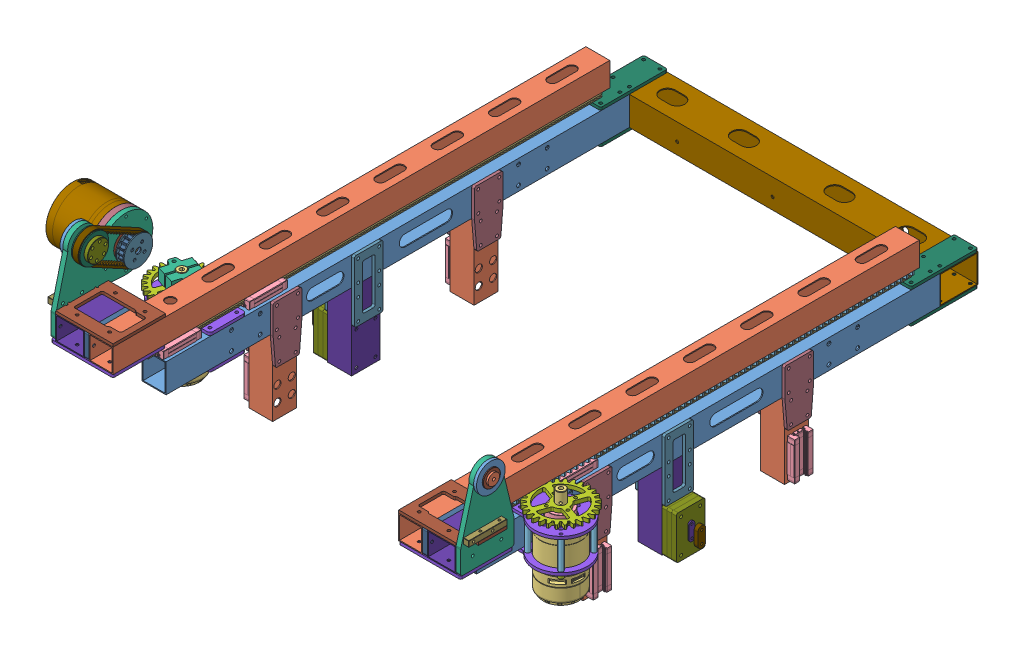
SolidWorks assembly 前探2.0, configuration 默认. Lengths in mm. (continued)
Mates (geometry in assembly coordinates): (continued)
- 同心473: concentric anti-aligned: cylinder of 12.9级圆柱头螺钉-18 through (155 19 124.65) axis (0 1 0) radius 1.5; cylinder of 上银直线导轨线性滑轨MGN-C-O╱MGN-H-O[MGN9H2R475ZACI＋-O]_1-4 through (155 15 124.65) axis (0 -1 0) radius 1.5
- 同心474: concentric anti-aligned: cylinder of 12.9级圆柱头螺钉-16 through (155 19 140.65) axis (0 1 0) radius 1.5; cylinder of 上银直线导轨线性滑轨MGN-C-O╱MGN-H-O[MGN9H2R475ZACI＋-O]_1-4 through (155 15 140.65) axis (0 -1 0) radius 1.5
- 同心475: concentric anti-aligned: cylinder of 12.9级圆柱头螺钉-17 through (170 19 124.65) axis (0 1 0) radius 1.5; cylinder of 上银直线导轨线性滑轨MGN-C-O╱MGN-H-O[MGN9H2R475ZACI＋-O]_1-4 through (170 15 124.65) axis (0 -1 0) radius 1.5
- 重合8072: coincident aligned: plane of 横移连接板-2 through (123.1167 31 299) normal (0 0 1); plane of 25x30x1铝方管-2 through (195 43.5 299) normal (0 0 1)
- 重合8076: coincident anti-aligned: plane of 25x25x1铝方管-1 through (-175 31 298) normal (0 -1 0); plane of 齿条2X76-1 through (158 31 244) normal (0 1 0)
- 平行9: parallel aligned: plane of 25x25x1铝方管-2 through (150 31 299) normal (-1 0 0); plane of 齿条2X76-1 through (158 25 244) normal (-1 0 0)
- 重合8077: coincident aligned: plane of 25x25x1铝方管-2 through (162.5 43.5 -221) normal (0 0 -1); plane of 齿条2X76-1 through (168 25 -221) normal (0 0 -1)
- 重合8078: coincident aligned: plane of 上银直线导轨线性滑轨MGN-C-O╱MGN-H-O[MGN9H2R475ZACI＋-O]_2-2 through (158 24.6775 254) normal (-1 0 0); plane of 齿条2X76-1 through (158 25 244) normal (-1 0 0)
- 重合8080: coincident anti-aligned: plane of 25x25x1铝方管-1 through (-175 31 298) normal (0 -1 0); plane of 齿条2X76-3 through (-158 31 243) normal (0 1 0)
- 重合8081: coincident aligned: plane of 上银直线导轨线性滑轨MGN-C-O╱MGN-H-O[MGN9H2R475ZACI＋-O]_2-1 through (-158 24.6775 253) normal (1 0 0); plane of 齿条2X76-3 through (-158 31 243) normal (1 0 0)
- 重合8082: coincident aligned: plane of 上银直线导轨线性滑轨MGN-C-O╱MGN-H-O[MGN9H2R475ZACI＋-O]_2-1 through (-157.775 20.65 -222) normal (0 0 -1); plane of 齿条2X76-3 through (-168 31 -222) normal (0 0 -1)
- 同心476: concentric anti-aligned: cylinder of RoboMaster M3508直流无刷减速电机-1 through (-198.5 42.3 177.6) axis (0 1 0) radius 5; cylinder of 2孔夹紧联轴器-1 through (-198.5 42 177.6) axis (0 -1 0) radius 5
- 距离22: distance = 26 mm: cylinder of 圆柱齿轮28×2-1 through (-198.5 31 177.6) axis (0 -1 0) radius 5; plane of 齿条2X76-3 through (-172.5 18.3018 -85.3635) normal (-1 0 0)
- 宽度26: width aligned: plane of 齿条2X76-3 through (-158 31 243) normal (0 1 0); plane of 圆柱齿轮28×2-1 through (-158 25 243) normal (0 -1 0); plane of 齿条2X76-3 through (-198.5 30 177.6) normal (0 1 0); plane of 圆柱齿轮28×2-1 through (-198.5 26 177.6) normal (0 -1 0)
- 同心478: concentric anti-aligned: cylinder of RoboMaster M3508直流无刷减速电机-1 through (-198.5 42.3 177.6) axis (0 1 0) radius 5; cylinder of 圆柱齿轮28×2-1 through (-198.5 31 177.6) axis (0 -1 0) radius 5
- 重合8086: coincident anti-aligned: plane of 推力球轴承-1 through (-198.5 26 177.6) normal (0 1 0); plane of 圆柱齿轮28×2-1 through (-198.5 26 177.6) normal (0 -1 0)
- 重合8087: coincident anti-aligned: plane of 2孔夹紧联轴器-1 through (-198.5 30 177.6) normal (0 -1 0); plane of 圆柱齿轮28×2-1 through (-198.5 30 177.6) normal (0 1 0)
- 重合8088: coincident anti-aligned: plane of 30x25x1铝方管-6 through (-175 15 242.5) normal (0 1 0); plane of 前探3508安装板-1 through (-198.5 15 177.6) normal (0 -1 0)
- 同心479: concentric anti-aligned: cylinder of RoboMaster M3508直流无刷减速电机-1 through (-198.5 34.1192 177.6) axis (0 1 0) radius 21; cylinder of 前探3508安装板-1 through (-198.5 18 177.6) axis (0 -1 0) radius 27.5
- 宽度28: width anti-aligned: plane of 上银直线导轨线性滑轨MGN-C-O╱MGN-H-O[MGN9H2R475ZACI＋-O]_1-2 through (-162.5 32.2555 152.6) normal (0 0 1); plane of 前探3508安装板-1 through (-162.5 32.2555 202.6) normal (0 0 -1); plane of 上银直线导轨线性滑轨MGN-C-O╱MGN-H-O[MGN9H2R475ZACI＋-O]_1-1 through (-150 -32.5716 158.6) normal (0 0 -1); plane of 前探3508安装板-1 through (-178.6191 -32.5716 196.6) normal (0 0 1)
- 同心480: concentric anti-aligned: cylinder of 304不锈钢接线柱-4 through (-181.1759 15 160.2759) axis (0 1 0) radius 2.5; cylinder of 前探3508安装板-1 through (-181.1759 22.3134 160.2759) axis (0 -1 0) radius 1.525
- 重合8089: coincident anti-aligned: plane of 304不锈钢接线柱-4 through (-179.2918 15 161.9191) normal (0 1 0); plane of 前探3508安装板-1 through (-198.5 15 177.6) normal (0 -1 0)
- 重合8090: coincident anti-aligned: plane of 304不锈钢接线柱-1 through (-213.3243 15 160.2444) normal (0 1 0); plane of 前探3508安装板-1 through (-198.5 15 177.6) normal (0 -1 0)
- 同心481: concentric anti-aligned: cylinder of 304不锈钢接线柱-1 through (-215.8241 15 160.2759) axis (0 1 0) radius 2.5; cylinder of 前探3508安装板-1 through (-215.8241 22.3134 160.2759) axis (0 -1 0) radius 1.525
- 同心482: concentric anti-aligned: cylinder of 304不锈钢接线柱-4 through (-181.1759 -15 160.2759) axis (0 -1 0) radius 1.25; cylinder of 12.9级圆柱头螺钉-4 through (-181.1759 -10 160.2759) axis (0 1 0) radius 1.5
- 同心483: concentric anti-aligned: cylinder of 304不锈钢接线柱-1 through (-215.8241 -15 160.2759) axis (0 -1 0) radius 1.25; cylinder of 12.9级圆柱头螺钉-3 through (-215.8241 -10 160.2759) axis (0 1 0) radius 1.5
- 重合8091: coincident anti-aligned: plane of 30x25x1铝方管-2 through (150 15 242.5) normal (0 1 0); plane of 前探3508安装板-2 through (198.5 15 177.6) normal (0 -1 0)
- 宽度29: width anti-aligned: plane of 上银直线导轨线性滑轨MGN-C-O╱MGN-H-O[MGN9H2R475ZACI＋-O]_1-4 through (162.5 32.2555 152.6) normal (0 0 1); plane of 前探3508安装板-2 through (162.5 32.2555 202.6) normal (0 0 -1); plane of 上银直线导轨线性滑轨MGN-C-O╱MGN-H-O[MGN9H2R475ZACI＋-O]_1-3 through (150 65.5716 158.6) normal (0 0 -1); plane of 前探3508安装板-2 through (178.6191 65.5716 196.6) normal (0 0 1)
- 同心484: concentric anti-aligned: cylinder of RoboMaster M3508直流无刷减速电机-2 through (198.5 42.3 177.6) axis (0 1 0) radius 5; cylinder of 圆柱齿轮28×2-2 through (198.5 31 177.6) axis (0 -1 0) radius 5
- 重合8092: coincident anti-aligned: plane of 推力球轴承-2 through (198.5 26 177.6) normal (0 1 0); plane of 圆柱齿轮28×2-2 through (198.5 26 177.6) normal (0 -1 0)
- 同心485: concentric anti-aligned: cylinder of RoboMaster M3508直流无刷减速电机-2 through (198.5 42.3 177.6) axis (0 1 0) radius 5; cylinder of 2孔夹紧联轴器-2 through (198.5 42 177.6) axis (0 -1 0) radius 5
- 重合8093: coincident anti-aligned: plane of 2孔夹紧联轴器-2 through (210.7651 30 175.0373) normal (0 -1 0); plane of 圆柱齿轮28×2-2 through (198.5 30 177.6) normal (0 1 0)
- 距离23: distance = 26 mm: cylinder of 圆柱齿轮28×2-2 through (198.5 -1.2931 177.6) axis (0 1 0) radius 9; plane of 齿条2X76-1 through (172.5 37.6982 160.6807) normal (1 0 0)
- 同心486: concentric aligned: cylinder of RoboMaster M3508直流无刷减速电机-2 through (198.5 34.1192 177.6) axis (0 1 0) radius 21; cylinder of 前探3508安装板-2 through (198.5 15 177.6) axis (0 1 0) radius 27.5
- 同心487: concentric aligned: cylinder of 304不锈钢接线柱-6 through (215.8241 15 194.9241) axis (0 1 0) radius 2.5; cylinder of 前探3508安装板-2 through (215.8241 10.6866 194.9241) axis (0 1 0) radius 1.525
- 重合8094: coincident anti-aligned: plane of 304不锈钢接线柱-6 through (218.0092 15 196.1389) normal (0 1 0); plane of 前探3508安装板-2 through (198.5 15 177.6) normal (0 -1 0)
- 同心488: concentric aligned: cylinder of 304不锈钢接线柱-5 through (215.8241 15 160.2759) axis (0 1 0) radius 2.5; cylinder of 前探3508安装板-2 through (215.8241 10.6866 160.2759) axis (0 1 0) radius 1.525
- 重合8095: coincident anti-aligned: plane of 304不锈钢接线柱-5 through (218.1812 15 161.109) normal (0 1 0); plane of 前探3508安装板-2 through (198.5 15 177.6) normal (0 -1 0)
- 同心489: concentric aligned: cylinder of 304不锈钢接线柱-8 through (181.1759 15 160.2759) axis (0 1 0) radius 2.5; cylinder of 前探3508安装板-2 through (181.1759 10.6866 160.2759) axis (0 1 0) radius 1.525
- 重合8096: coincident anti-aligned: plane of 304不锈钢接线柱-8 through (183.6584 15 160.5708) normal (0 1 0); plane of 前探3508安装板-2 through (198.5 15 177.6) normal (0 -1 0)
- 同心490: concentric anti-aligned: cylinder of 304不锈钢接线柱-6 through (215.8241 -15 194.9241) axis (0 -1 0) radius 1.25; cylinder of 12.9级圆柱头螺钉-7 through (215.8241 -10 194.9241) axis (0 1 0) radius 1.5
- 同心491: concentric anti-aligned: cylinder of 304不锈钢接线柱-5 through (215.8241 -15 160.2759) axis (0 -1 0) radius 1.25; cylinder of 12.9级圆柱头螺钉-6 through (215.8241 -10 160.2759) axis (0 1 0) radius 1.5
- 同心492: concentric anti-aligned: cylinder of 304不锈钢接线柱-8 through (181.1759 -15 160.2759) axis (0 -1 0) radius 1.25; cylinder of 12.9级圆柱头螺钉-5 through (181.1759 -10 160.2759) axis (0 1 0) radius 1.5
- 距离24: distance = 300 mm anti-aligned: plane of 30x25x1铝方管-6 through (-150 -15 242.5) normal (1 0 0); plane of 30x25x1铝方管-2 through (150 -15 242.5) normal (-1 0 0)
- 同心493: concentric anti-aligned: cylinder of 304不锈钢接线柱-3 through (-215.8241 15 194.9241) axis (0 1 0) radius 2.5; cylinder of 前探3508安装板-1 through (-215.8241 22.3134 194.9241) axis (0 -1 0) radius 1.525
- 重合8097: coincident anti-aligned: plane of 304不锈钢接线柱-3 through (-213.467 15 195.7572) normal (0 1 0); plane of 前探3508安装板-1 through (-198.5 15 177.6) normal (0 -1 0)
- 同心494: concentric anti-aligned: cylinder of 304不锈钢接线柱-3 through (-215.8241 -15 194.9241) axis (0 -1 0) radius 1.25; cylinder of 12.9级圆柱头螺钉-2 through (-215.8241 -10 194.9241) axis (0 1 0) radius 1.5
- 重合8098: coincident anti-aligned: plane of 30x25x1铝方管-2 through (162.5 0 -242.5) normal (0 0 -1); plane of 40x30x1铝方管-1 through (-175 -15 -242.5) normal (0 0 1)
- 重合8099: coincident aligned: plane of 30x25x1铝方管-2 through (150 -15 242.5) normal (0 -1 0); plane of 40x30x1铝方管-1 through (-175 -15 -282.5) normal (0 -1 0)
- 重合8100: coincident aligned: plane of 30x25x1铝方管-2 through (175 -15 242.5) normal (1 0 0); plane of 40x30x1铝方管-1 through (175 0 -262.5) normal (1 0 0)
- 重合8101: coincident anti-aligned: plane of 30x25x1铝方管-6 through (-162.5 0 -242.5) normal (0 0 -1); plane of 40x30x1铝方管-1 through (-175 -15 -242.5) normal (0 0 1)
- 距离27: distance = 861 mm: cylinder of 转点垫片-1 through (-221.1 108 270.5) axis (1 0 0) radius 6; plane of 40x30x1铝方管-1 through (-175 -15 -282.5) normal (0 0 -1)
- LimitDistance1: limit distance = 60.5 mm aligned: plane of 40x30x1铝方管-1 through (-175 -15 -282.5) normal (0 0 -1); plane of 上银直线导轨线性滑轨MGN-C-O╱MGN-H-O[MGN9H2R475ZACI＋-O]_2-1 through (-157.775 20.65 -222) normal (0 0 -1)
- 重合8105: coincident anti-aligned: plane of RoboMaster M3508直流无刷减速电机-2 through (197.8369 15 190.5831) normal (0 1 0); plane of 前探3508安装板-2 through (198.5 15 177.6) normal (0 -1 0)
- 重合8106: coincident anti-aligned: plane of 30x25x1铝方管-6 through (-175 -15 242.5) normal (0 -1 0); plane of 前探3508安装板-3 through (-198.5 -15 177.6) normal (0 1 0)
- 同心495: concentric anti-aligned: cylinder of RoboMaster M3508直流无刷减速电机-1 through (-198.5 -21 177.6) axis (0 -1 0) radius 21; cylinder of 前探3508安装板-3 through (-198.5 -30 177.6) axis (0 1 0) radius 21.5
- 平行10: parallel aligned: plane of 30x25x1铝方管-6 through (-150 -15 242.5) normal (1 0 0); plane of 前探3508安装板-3 through (-150 -65.5716 196.6) normal (1 0 0)
- 重合8107: coincident anti-aligned: plane of 12.9级圆柱头螺钉-2 through (-212.9858 -18 194.8255) normal (0 1 0); plane of 前探3508安装板-3 through (-198.5 -18 177.6) normal (0 -1 0)
- 重合8108: coincident anti-aligned: plane of 12.9级圆柱头螺钉-3 through (-214.0645 -18 158.0467) normal (0 1 0); plane of 前探3508安装板-3 through (-198.5 -18 177.6) normal (0 -1 0)
- 重合8109: coincident anti-aligned: plane of 12.9级圆柱头螺钉-4 through (-179.8982 -18 162.8122) normal (0 1 0); plane of 前探3508安装板-3 through (-198.5 -18 177.6) normal (0 -1 0)
- 同心496: concentric anti-aligned: cylinder of 前探3508安装板-1 through (-181.1759 22.3134 194.9241) axis (0 -1 0) radius 1.525; cylinder of 304不锈钢接线柱-9 through (-181.1759 15 194.9241) axis (0 1 0) radius 2.5
- 重合8110: coincident anti-aligned: plane of 前探3508安装板-1 through (-198.5 15 177.6) normal (0 -1 0); plane of 304不锈钢接线柱-9 through (-178.6759 15 194.9252) normal (0 1 0)
- 同心4971: concentric anti-aligned: cylinder of 前探3508安装板-3 through (-181.1759 -10.6866 194.9241) axis (0 -1 0) radius 1.525; cylinder of 12.9级圆柱头螺钉-27 through (-181.1759 -10 194.9241) axis (0 1 0) radius 2.84
- 重合81111: coincident anti-aligned: plane of 前探3508安装板-3 through (-198.5 -18 177.6) normal (0 -1 0); plane of 12.9级圆柱头螺钉-27 through (-178.3376 -18 194.8255) normal (0 1 0)
- 同心498: concentric aligned: cylinder of RoboMaster M3508直流无刷减速电机-2 through (198.5 -21 177.6) axis (0 -1 0) radius 21; cylinder of 前探3508安装板-4 through (198.5 -3 177.6) axis (0 -1 0) radius 21.5
- 平行11: parallel aligned: plane of 30x25x1铝方管-2 through (150 -15 242.5) normal (-1 0 0); plane of 前探3508安装板-4 through (150 32.5716 196.6) normal (-1 0 0)
- 重合8112: coincident anti-aligned: plane of 30x25x1铝方管-2 through (150 -15 242.5) normal (0 -1 0); plane of 前探3508安装板-4 through (198.5 -15 177.6) normal (0 1 0)
- 同心500: concentric aligned: cylinder of 304不锈钢接线柱-7 through (181.1759 15 194.9241) axis (0 1 0) radius 2.5; cylinder of 前探3508安装板-4 through (181.1759 -22.3134 194.9241) axis (0 1 0) radius 1.525
- 同心501: concentric aligned: cylinder of 304不锈钢接线柱-7 through (181.1759 15 194.9241) axis (0 1 0) radius 2.5; cylinder of 12.9级圆柱头螺钉-8 through (181.1759 -10 194.9241) axis (0 1 0) radius 1.5
- 重合8113: coincident anti-aligned: plane of 12.9级圆柱头螺钉-8 through (181.3223 -18 197.7603) normal (0 1 0); plane of 前探3508安装板-4 through (198.5 -18 177.6) normal (0 -1 0)
- 重合8114: coincident anti-aligned: plane of 304不锈钢接线柱-7 through (181.1759 -15 194.9241) normal (0 -1 0); plane of 前探3508安装板-4 through (198.5 -15 177.6) normal (0 1 0)
- 重合8115: coincident anti-aligned: plane of 12.9级圆柱头螺钉-5 through (180.983 -18 163.1093) normal (0 1 0); plane of 前探3508安装板-4 through (198.5 -18 177.6) normal (0 -1 0)
- 重合8116: coincident anti-aligned: plane of 12.9级圆柱头螺钉-6 through (215.2807 -18 163.0634) normal (0 1 0); plane of 前探3508安装板-4 through (198.5 -18 177.6) normal (0 -1 0)
- 重合8117: coincident anti-aligned: plane of 12.9级圆柱头螺钉-7 through (215.9108 -18 197.7628) normal (0 1 0); plane of 前探3508安装板-4 through (198.5 -18 177.6) normal (0 -1 0)
- 距离28: distance = 5 mm anti-aligned: plane of 25x30x1铝方管-1 through (-180 31 298) normal (1 0 0); plane of 25x25x1铝方管-1 through (-175 31 298) normal (-1 0 0)
- 距离29: distance = 5 mm anti-aligned: plane of 25x30x1铝方管-2 through (180 31 299) normal (-1 0 0); plane of 25x25x1铝方管-2 through (175 31 299) normal (1 0 0)
- 重合81115: coincident aligned: plane of 30x25x1铝方管-2 through (150 -15 242.5) normal (-1 0 0); plane of 25x25x1铝方管-3 through (150 -95 105.9) normal (-1 0 0)
- 重合81116: coincident anti-aligned: plane of 30x25x1铝方管-2 through (150 -15 242.5) normal (0 -1 0); plane of 25x25x1铝方管-3 through (162.5 -15 118.4) normal (0 1 0)
- 重合81117: coincident anti-aligned: line of 30x25x1铝方管-2 through (150 15 130.9) axis (0 -1 0); line of 25x25x1铝方管-3 through (150 -95 130.9) axis (0 1 0)
- 重合81118: coincident anti-aligned: plane of 30x25x1铝方管-2 through (150 -15 242.5) normal (0 -1 0); plane of 25x25x1铝方管-4 through (162.5 -15 -92.4) normal (0 1 0)
- 重合81119: coincident aligned: plane of 30x25x1铝方管-2 through (150 -15 242.5) normal (-1 0 0); plane of 25x25x1铝方管-4 through (150 -95 -104.9) normal (-1 0 0)
- 重合81120: coincident: point of 30x25x1铝方管-2; plane of 25x25x1铝方管-4 through (150 -95 -104.9) normal (0 0 -1)
- 重合81121: coincident anti-aligned: plane of 25x25x1铝方管-3 through (175 -95 105.9) normal (1 0 0); plane of 上银直线导轨线性滑轨MGN-C-O╱MGN-H-O[MGN9H2R475ZACI＋-O]_1-5 through (175 -57.4 128.4) normal (-1 0 0)
- 宽度30: width aligned: plane of 25x25x1铝方管-3 through (150 -95 130.9) normal (0 0 1); plane of 25x25x1铝方管-3 through (150 -95 105.9) normal (0 0 -1); plane of 上银直线导轨线性滑轨MGN-C-O╱MGN-H-O[MGN9H2R475ZACI＋-O]_1-5 through (177 -57.4 128.4) normal (0 0 1); plane of 上银直线导轨线性滑轨MGN-C-O╱MGN-H-O[MGN9H2R475ZACI＋-O]_1-5 through (177 -57.4 108.4) normal (0 0 -1)
- 距离30: distance = 3 mm aligned: plane of 上银直线导轨线性滑轨MGN-C-O╱MGN-H-O[MGN9H2R475ZACI＋-O]_1-5 through (192.2555 -92 118.4) normal (0 -1 0); plane of 25x25x1铝方管-3 through (162.5 -95 118.4) normal (0 -1 0)
- 重合81122: coincident aligned: plane of 上银直线导轨线性滑轨MGN-C-O╱MGN-H-O[MGN9H2R475ZACI＋-O]_1-5 through (192.2555 -92 118.4) normal (0 -1 0); plane of 上银直线导轨线性滑轨MGN-C-O╱MGN-H-O[MGN9H2R475ZACI＋-O]_1-6 through (192.2555 -92 -92.4) normal (0 -1 0)
- 重合81123: coincident anti-aligned: plane of 25x25x1铝方管-4 through (175 -95 -104.9) normal (1 0 0); plane of 上银直线导轨线性滑轨MGN-C-O╱MGN-H-O[MGN9H2R475ZACI＋-O]_1-6 through (175 -57.4 -82.4) normal (-1 0 0)
- 宽度31: width aligned: plane of 25x25x1铝方管-4 through (150 -95 -79.9) normal (0 0 1); plane of 25x25x1铝方管-4 through (150 -95 -104.9) normal (0 0 -1); plane of 上银直线导轨线性滑轨MGN-C-O╱MGN-H-O[MGN9H2R475ZACI＋-O]_1-6 through (177 -57.4 -82.4) normal (0 0 1); plane of 上银直线导轨线性滑轨MGN-C-O╱MGN-H-O[MGN9H2R475ZACI＋-O]_1-6 through (177 -57.4 -102.4) normal (0 0 -1)
- 重合81124: coincident aligned: plane of 30x25x1铝方管-6 through (-150 -15 242.5) normal (1 0 0); plane of 25x25x1铝方管-5 through (-150 -95 130.9) normal (1 0 0)
- 重合81125: coincident anti-aligned: plane of 30x25x1铝方管-6 through (-175 -15 242.5) normal (0 -1 0); plane of 25x25x1铝方管-5 through (-162.5 -15 118.4) normal (0 1 0)
- 重合81126: coincident: plane of 30x25x1铝方管-6; plane of 25x25x1铝方管-5 through (-150 -95 130.9) normal (0 0 1)
- 重合81127: coincident anti-aligned: plane of 30x25x1铝方管-6 through (-175 -15 242.5) normal (0 -1 0); plane of 25x25x1铝方管-6 through (-162.5 -15 -92.4) normal (0 1 0)
- 重合81128: coincident aligned: plane of 30x25x1铝方管-6 through (-175 -15 242.5) normal (-1 0 0); plane of 25x25x1铝方管-6 through (-175 -95 -79.9) normal (-1 0 0)
- 重合81129: coincident anti-aligned: line of 30x25x1铝方管-6 through (-175 15 -79.9) axis (0 -1 0); line of 25x25x1铝方管-6 through (-175 -95 -79.9) axis (0 1 0)
- 重合81130: coincident anti-aligned: plane of 25x25x1铝方管-6 through (-175 -95 -79.9) normal (-1 0 0); plane of 上银直线导轨线性滑轨MGN-C-O╱MGN-H-O[MGN9H2R475ZACI＋-O]_1-7 through (-175 -86.7 -82.4) normal (1 0 0)
- 宽度32: width aligned: plane of 25x25x1铝方管-6 through (-150 -95 -104.9) normal (0 0 -1); plane of 25x25x1铝方管-6 through (-150 -95 -79.9) normal (0 0 1); plane of 上银直线导轨线性滑轨MGN-C-O╱MGN-H-O[MGN9H2R475ZACI＋-O]_1-7 through (-177 -86.7 -102.4) normal (0 0 -1); plane of 上银直线导轨线性滑轨MGN-C-O╱MGN-H-O[MGN9H2R475ZACI＋-O]_1-7 through (-177 -86.7 -82.4) normal (0 0 1)
- 宽度33: width aligned: plane of 25x25x1铝方管-5 through (-150 -95 105.9) normal (0 0 -1); plane of 25x25x1铝方管-5 through (-150 -95 130.9) normal (0 0 1); plane of 上银直线导轨线性滑轨MGN-C-O╱MGN-H-O[MGN9H2R475ZACI＋-O]_1-8 through (-177 -86.7 108.4) normal (0 0 -1); plane of 上银直线导轨线性滑轨MGN-C-O╱MGN-H-O[MGN9H2R475ZACI＋-O]_1-8 through (-177 -86.7 128.4) normal (0 0 1)
- 重合81131: coincident anti-aligned: plane of 25x25x1铝方管-5 through (-175 -95 130.9) normal (-1 0 0); plane of 上银直线导轨线性滑轨MGN-C-O╱MGN-H-O[MGN9H2R475ZACI＋-O]_1-8 through (-175 -86.7 128.4) normal (1 0 0)
- 重合81132: coincident aligned: plane of 上银直线导轨线性滑轨MGN-C-O╱MGN-H-O[MGN9H2R475ZACI＋-O]_1-7 through (-192.2555 -92 -92.4) normal (0 -1 0); plane of 上银直线导轨线性滑轨MGN-C-O╱MGN-H-O[MGN9H2R475ZACI＋-O]_1-8 through (-192.2555 -92 118.4) normal (0 -1 0)
- 重合81133: coincident aligned: plane of 上银直线导轨线性滑轨MGN-C-O╱MGN-H-O[MGN9H2R475ZACI＋-O]_1-6 through (192.2555 -92 -92.4) normal (0 -1 0); plane of 上银直线导轨线性滑轨MGN-C-O╱MGN-H-O[MGN9H2R475ZACI＋-O]_1-7 through (-192.2555 -92 -92.4) normal (0 -1 0)
- 重合81134: coincident anti-aligned: plane of 25x25x1铝方管-1 through (-175 31 298) normal (-1 0 0); plane of 前探垫块-1 through (-175 43.5 270.5) normal (1 0 0)
- 重合81135: coincident anti-aligned: plane of 支撑连接板-2 through (-182.5 31 270.5) normal (0 1 0); plane of 前探垫块-1 through (-175 31 298) normal (0 -1 0)
- 重合81136: coincident aligned: plane of 25x30x1铝方管-1 through (-195 43.5 298) normal (0 0 1); plane of 前探垫块-1 through (-175 31 298) normal (0 0 1)
- 重合81137: coincident aligned: plane of 25x30x1铝方管-2 through (195 43.5 299) normal (0 0 1); plane of 前探垫块-2 through (180 31 299) normal (0 0 1)
- 重合81138: coincident anti-aligned: plane of 25x30x1铝方管-2 through (180 31 299) normal (-1 0 0); plane of 前探垫块-2 through (180 43.5 271.5) normal (1 0 0)
- 重合81139: coincident aligned: plane of 25x30x1铝方管-2 through (180 56 299) normal (0 1 0); plane of 前探垫块-2 through (180 56 299) normal (0 1 0)
- 重合81140: coincident anti-aligned: plane of 25x25x1铝方管-1 through (-175 56 298) normal (0 1 0); plane of 前探加固板-1 through (-180 56 270.5) normal (0 -1 0)
- 重合81141: coincident aligned: plane of 25x30x1铝方管-1 through (-195 43.5 298) normal (0 0 1); plane of 前探加固板-1 through (-150 56 298) normal (0 0 1)
- 重合81142: coincident anti-aligned: plane of 横移连接板-1 through (-210 43.5 263) normal (1 0 0); plane of 前探加固板-1 through (-210 56 243) normal (-1 0 0)
- 重合81143: coincident anti-aligned: plane of 前探加固板-1 through (-180 59 270.5) normal (0 1 0); plane of 四孔直角转接件-1 through (-215 59 295.5) normal (0 -1 0)
- 重合81144: coincident anti-aligned: plane of 横移连接板-1 through (-215 43.5 263) normal (-1 0 0); plane of 四孔直角转接件-1 through (-215 59 295.5) normal (1 0 0)
- 重合81145: coincident aligned: plane of 前探加固板-1 through (-199 18.7978 255.5) normal (0 0 -1); plane of 四孔直角转接件-1 through (-218 62 255.5) normal (0 0 -1)
- 重合81146: coincident anti-aligned: plane of 25x30x1铝方管-2 through (180 56 299) normal (0 1 0); plane of 前探加固板-2 through (180 56 271.5) normal (0 -1 0)
- 重合81147: coincident aligned: plane of 前探垫块-2 through (180 31 299) normal (0 0 1); plane of 前探加固板-2 through (150 59 299) normal (0 0 1)
- 重合81148: coincident anti-aligned: plane of 横移连接板-2 through (210 43.5 263) normal (-1 0 0); plane of 前探加固板-2 through (210 59 244) normal (1 0 0)
- 重合81149: coincident anti-aligned: plane of 前探加固板-2 through (180 59 271.5) normal (0 1 0); plane of 四孔直角转接件-2 through (221 59 296.5) normal (0 -1 0)
- 重合81150: coincident aligned: plane of 前探加固板-2 through (199 96.2022 256.5) normal (0 0 -1); plane of 四孔直角转接件-2 through (218 62 256.5) normal (0 0 -1)
- 重合81151: coincident anti-aligned: plane of 横移连接板-2 through (215 43.5 263) normal (1 0 0); plane of 四孔直角转接件-2 through (215 59 296.5) normal (-1 0 0)
- 重合81152: coincident aligned: plane of 30x25x1铝方管-6 through (-175 -15 242.5) normal (-1 0 0); plane of 25x30x1铝方管-3 through (-175 -15 18.295) normal (-1 0 0)
- 重合81153: coincident anti-aligned: plane of 30x25x1铝方管-6 through (-175 -15 242.5) normal (0 -1 0); plane of 25x30x1铝方管-3 through (-162.5 -15 33.295) normal (0 1 0)
- 距离31: distance = 15 mm: plane of 25x30x1铝方管-3 through (-175 -15 48.295) normal (0 0 1); line of 30x25x1铝方管-6 through (-175 15 33.295) axis (0 -1 0)
- 重合81154: coincident aligned: plane of 30x25x1铝方管-2 through (175 -15 242.5) normal (1 0 0); plane of 25x30x1铝方管-4 through (175 -15 48.295) normal (1 0 0)
- 重合81155: coincident anti-aligned: plane of 30x25x1铝方管-2 through (150 -15 242.5) normal (0 -1 0); plane of 25x30x1铝方管-4 through (162.5 -15 33.295) normal (0 1 0)
- 重合81156: coincident aligned: plane of 25x30x1铝方管-3 through (-175 -15 48.295) normal (0 0 1); plane of 25x30x1铝方管-4 through (175 -15 48.295) normal (0 0 1)
- 重合81157: coincident anti-aligned: plane of 25x25x1铝方管-6 through (-175 -95 -79.9) normal (-1 0 0); plane of 抬升连接板1-1 through (-175 0 -92.4) normal (1 0 0)
- 重合81158: coincident aligned: plane of 30x25x1铝方管-6 through (-175 15 242.5) normal (0 1 0); plane of 抬升连接板1-1 through (-178 15 -92.4) normal (0 1 0)
- 宽度34: width aligned: plane of 抬升连接板1-1 through (-178 0 -77.4) normal (0 0 1); plane of 抬升连接板1-1 through (-178 0 -107.4) normal (0 0 -1); plane of 25x25x1铝方管-6 through (-150 -95 -79.9) normal (0 0 1); plane of 25x25x1铝方管-6 through (-150 -95 -104.9) normal (0 0 -1)
- 重合811591: coincident anti-aligned: plane of 25x25x1铝方管-5 through (-175 -95 130.9) normal (-1 0 0); plane of 抬升连接板1-2 through (-175 0 118.4) normal (1 0 0)
- 重合81160: coincident aligned: plane of 30x25x1铝方管-6 through (-175 15 242.5) normal (0 1 0); plane of 抬升连接板1-2 through (-175 15 118.4) normal (0 1 0)
- 宽度35: width aligned: plane of 抬升连接板1-2 through (-175 0 103.4) normal (0 0 -1); plane of 抬升连接板1-2 through (-175 0 133.4) normal (0 0 1); plane of 25x25x1铝方管-5 through (-150 -95 105.9) normal (0 0 -1); plane of 25x25x1铝方管-5 through (-150 -95 130.9) normal (0 0 1)
- 重合81161: coincident anti-aligned: plane of 25x25x1铝方管-6 through (-150 -95 -79.9) normal (1 0 0); plane of 抬升连接板1-3 through (-150 0 -92.4) normal (-1 0 0)
- 重合81162: coincident aligned: plane of 30x25x1铝方管-6 through (-175 15 242.5) normal (0 1 0); plane of 抬升连接板1-3 through (-150 15 -92.4) normal (0 1 0)
- 重合811631: coincident anti-aligned: plane of 25x30x1铝方管-3 through (-150 -15 18.295) normal (1 0 0); plane of 抬升连接板1-4 through (-150 0 118.4) normal (-1 0 0)
- 宽度36: width aligned: plane of 抬升连接板1-4 through (-147 0 103.4) normal (0 0 -1); plane of 抬升连接板1-4 through (-147 0 133.4) normal (0 0 1); plane of 25x25x1铝方管-5 through (-150 -95 105.9) normal (0 0 -1); plane of 25x25x1铝方管-5 through (-150 -95 130.9) normal (0 0 1)
- 重合81164: coincident aligned: plane of 抬升连接板1-2 through (-175 15 118.4) normal (0 1 0); plane of 抬升连接板1-4 through (-147 15 118.4) normal (0 1 0)
- 宽度37: width aligned: plane of 抬升连接板1-3 through (-150 0 -77.4) normal (0 0 1); plane of 抬升连接板1-3 through (-150 0 -107.4) normal (0 0 -1); plane of 25x25x1铝方管-6 through (-150 -95 -79.9) normal (0 0 1); plane of 25x25x1铝方管-6 through (-150 -95 -104.9) normal (0 0 -1)
- 重合81165: coincident anti-aligned: plane of 30x25x1铝方管-6 through (-175 -15 242.5) normal (-1 0 0); plane of 抬升连接板2-1 through (-175 -17.5 33.295) normal (1 0 0)
- 重合81166: coincident aligned: plane of 30x25x1铝方管-6 through (-175 15 242.5) normal (0 1 0); plane of 抬升连接板2-1 through (-178 15 18.295) normal (0 1 0)
- 重合81167: coincident aligned: plane of 25x30x1铝方管-3 through (-175 -15 18.295) normal (0 0 -1); plane of 抬升连接板2-1 through (-178 -50 18.295) normal (0 0 -1)
- 重合81168: coincident anti-aligned: plane of 25x30x1铝方管-3 through (-150 -15 18.295) normal (1 0 0); plane of 抬升连接板2-2 through (-150 -17.5 33.295) normal (-1 0 0)
- 重合81169: coincident aligned: plane of 25x30x1铝方管-3 through (-175 -15 18.295) normal (0 0 -1); plane of 抬升连接板2-2 through (-150 -50 18.295) normal (0 0 -1)
- 重合81170: coincident aligned: plane of 30x25x1铝方管-6 through (-175 15 242.5) normal (0 1 0); plane of 抬升连接板2-2 through (-150 15 18.295) normal (0 1 0)
- 重合81171: coincident anti-aligned: plane of 30x25x1铝方管-2 through (175 -15 242.5) normal (1 0 0); plane of 抬升连接板1-5 through (175 0 118.4) normal (-1 0 0)
- 宽度38: width aligned: plane of 抬升连接板1-5 through (178 0 133.4) normal (0 0 1); plane of 抬升连接板1-5 through (178 0 103.4) normal (0 0 -1); plane of 25x25x1铝方管-3 through (150 -95 130.9) normal (0 0 1); plane of 25x25x1铝方管-3 through (150 -95 105.9) normal (0 0 -1)
- 重合81172: coincident aligned: plane of 30x25x1铝方管-2 through (150 15 242.5) normal (0 1 0); plane of 抬升连接板1-5 through (178 15 118.4) normal (0 1 0)
- 重合81173: coincident anti-aligned: plane of 25x25x1铝方管-3 through (150 -95 105.9) normal (-1 0 0); plane of 抬升连接板1-6 through (150 0 118.4) normal (1 0 0)
- 宽度39: width aligned: plane of 抬升连接板1-6 through (150 0 103.4) normal (0 0 -1); plane of 抬升连接板1-6 through (150 0 133.4) normal (0 0 1); plane of 25x25x1铝方管-3 through (150 -95 105.9) normal (0 0 -1); plane of 25x25x1铝方管-3 through (150 -95 130.9) normal (0 0 1)
- 重合81174: coincident aligned: plane of 30x25x1铝方管-2 through (150 15 242.5) normal (0 1 0); plane of 抬升连接板1-6 through (150 15 118.4) normal (0 1 0)
- 重合81175: coincident anti-aligned: plane of 30x25x1铝方管-2 through (175 -15 242.5) normal (1 0 0); plane of 抬升连接板1-7 through (175 0 -92.4) normal (-1 0 0)
- 宽度40: width aligned: plane of 抬升连接板1-7 through (178 0 -77.4) normal (0 0 1); plane of 抬升连接板1-7 through (178 0 -107.4) normal (0 0 -1); plane of 25x25x1铝方管-4 through (150 -95 -79.9) normal (0 0 1); plane of 25x25x1铝方管-4 through (150 -95 -104.9) normal (0 0 -1)
- 重合81176: coincident aligned: plane of 30x25x1铝方管-2 through (150 15 242.5) normal (0 1 0); plane of 抬升连接板1-7 through (178 15 -92.4) normal (0 1 0)
- 重合81177: coincident anti-aligned: plane of 30x25x1铝方管-2 through (150 -15 242.5) normal (-1 0 0); plane of 抬升连接板1-8 through (150 0 -92.4) normal (1 0 0)
- 重合81178: coincident aligned: plane of 30x25x1铝方管-2 through (150 15 242.5) normal (0 1 0); plane of 抬升连接板1-8 through (150 15 -92.4) normal (0 1 0)
- 宽度41: width aligned: plane of 抬升连接板1-8 through (150 0 -107.4) normal (0 0 -1); plane of 抬升连接板1-8 through (150 0 -77.4) normal (0 0 1); plane of 25x25x1铝方管-4 through (150 -95 -104.9) normal (0 0 -1); plane of 25x25x1铝方管-4 through (150 -95 -79.9) normal (0 0 1)
- 重合81179: coincident anti-aligned: plane of 30x25x1铝方管-2 through (175 -15 242.5) normal (1 0 0); plane of 抬升连接板2-3 through (175 -17.5 33.295) normal (-1 0 0)
- 重合81180: coincident aligned: plane of 25x30x1铝方管-4 through (175 -15 48.295) normal (0 0 1); plane of 抬升连接板2-3 through (175 -50 48.295) normal (0 0 1)
- 重合81181: coincident aligned: plane of 30x25x1铝方管-2 through (150 15 242.5) normal (0 1 0); plane of 抬升连接板2-3 through (175 15 18.295) normal (0 1 0)
- 重合81182: coincident anti-aligned: plane of 30x25x1铝方管-2 through (150 -15 242.5) normal (-1 0 0); plane of 抬升连接板2-4 through (150 -17.5 33.295) normal (1 0 0)
- 重合81183: coincident aligned: plane of 25x30x1铝方管-4 through (175 -15 48.295) normal (0 0 1); plane of 抬升连接板2-4 through (147 -50 48.295) normal (0 0 1)
- 重合81184: coincident aligned: plane of 30x25x1铝方管-2 through (150 15 242.5) normal (0 1 0); plane of 抬升连接板2-4 through (147 15 18.295) normal (0 1 0)
- 重合81185: coincident anti-aligned: plane of 40x30x1铝方管-1 through (-175 15 -282.5) normal (0 1 0); plane of 前探连接板-1 through (-162.5 15 -247.5) normal (0 -1 0)
- 重合81186: coincident aligned: plane of 40x30x1铝方管-1 through (-175 -15 -282.5) normal (0 0 -1); plane of 前探连接板-1 through (-150 18 -282.5) normal (0 0 -1)
- 重合81188: coincident aligned: plane of 30x25x1铝方管-6 through (-175 -15 242.5) normal (-1 0 0); plane of 前探连接板-1 through (-175 18 -212.5) normal (-1 0 0)
- 重合81189: coincident anti-aligned: plane of 40x30x1铝方管-1 through (-175 15 -282.5) normal (0 1 0); plane of 前探连接板-2 through (162.5 15 -247.5) normal (0 -1 0)
- 重合81191: coincident aligned: plane of 40x30x1铝方管-1 through (-175 -15 -282.5) normal (0 0 -1); plane of 前探连接板-2 through (175 18 -282.5) normal (0 0 -1)
- 重合81192: coincident aligned: plane of 40x30x1铝方管-1 through (175 0 -262.5) normal (1 0 0); plane of 前探连接板-2 through (175 18 -212.5) normal (1 0 0)
- 重合81193: coincident anti-aligned: plane of 40x30x1铝方管-1 through (-175 -15 -282.5) normal (0 -1 0); plane of 前探连接板-3 through (162.5 -15 -247.5) normal (0 1 0)
- 重合81194: coincident aligned: plane of 30x25x1铝方管-2 through (175 -15 242.5) normal (1 0 0); plane of 前探连接板-3 through (175 -15 -212.5) normal (1 0 0)
- 重合81195: coincident aligned: plane of 40x30x1铝方管-1 through (-175 -15 -282.5) normal (0 0 -1); plane of 前探连接板-3 through (175 -15 -282.5) normal (0 0 -1)
- 重合81196: coincident anti-aligned: plane of 40x30x1铝方管-1 through (-175 -15 -282.5) normal (0 -1 0); plane of 前探连接板-4 through (-162.5 -15 -247.5) normal (0 1 0)
- 重合81197: coincident aligned: plane of 30x25x1铝方管-6 through (-175 -15 242.5) normal (-1 0 0); plane of 前探连接板-4 through (-175 -15 -212.5) normal (-1 0 0)
- 重合81198: coincident aligned: plane of 40x30x1铝方管-1 through (-175 -15 -282.5) normal (0 0 -1); plane of 前探连接板-4 through (-150 -15 -282.5) normal (0 0 -1)
- 重合811632: coincident anti-aligned: plane of 25x30x1铝方管-3 through (-175 -15 18.295) normal (-1 0 0); plane of 抬升链条连接-1 through (-175 -72.5 33.295) normal (1 0 0)
- 重合811634: coincident aligned: plane of 25x30x1铝方管-3 through (-162.5 -95 33.295) normal (0 -1 0); plane of 抬升链条连接-1 through (-180 -95 18.295) normal (0 -1 0)
- 宽度42: width aligned: plane of 抬升链条连接-1 through (-180 -95 18.295) normal (0 0 -1); plane of 25x30x1铝方管-3 through (-180 -95 48.295) normal (0 0 1); plane of 抬升链条连接-1 through (-175 -15 18.295) normal (0 0 -1); plane of 25x30x1铝方管-3 through (-175 -15 48.295) normal (0 0 1)
- 重合811635: coincident anti-aligned: plane of 抬升链条连接-1 through (-180 -72.5 33.295) normal (-1 0 0); plane of 抬升链条连接-2 through (-180 -72.5 33.295) normal (1 0 0)
- 宽度43: width aligned: plane of 抬升链条连接-2 through (-185 -95 18.295) normal (0 0 -1); plane of 25x30x1铝方管-3 through (-185 -95 48.295) normal (0 0 1); plane of 抬升链条连接-2 through (-175 -15 18.295) normal (0 0 -1); plane of 25x30x1铝方管-3 through (-175 -15 48.295) normal (0 0 1)
- 重合811636: coincident aligned: plane of 抬升链条连接-1 through (-180 -95 18.295) normal (0 -1 0); plane of 抬升链条连接-2 through (-185 -95 18.295) normal (0 -1 0)
- 重合811637: coincident anti-aligned: plane of 上银直线导轨线性滑轨MGN-C-O╱MGN-H-O[MGN9H2R475ZACI＋-O]_2-1 through (-158.3225 25 253) normal (0 1 0); plane of 齿条2X76-3 through (-158 25 243) normal (0 -1 0)
- 重合811638: coincident anti-aligned: plane of 25x25x1铝方管-2 through (150 31 299) normal (0 -1 0); plane of 齿条2X76-1 through (158 31 244) normal (0 1 0)
- 重合811644: coincident aligned: plane of 抬升链条连接-2 through (-185 -95 18.295) normal (0 0 -1); plane of 抬升链条连接-5 through (-190 -95 18.295) normal (0 0 -1)
- 重合811646: coincident aligned: plane of 抬升链条连接-2 through (-185 -95 18.295) normal (0 -1 0); plane of 抬升链条连接-5 through (-190 -95 18.295) normal (0 -1 0)
- 重合811647: coincident anti-aligned: plane of 抬升链条连接-2 through (-185 -72.5 33.295) normal (-1 0 0); plane of 抬升链条连接-5 through (-185 -72.5 33.295) normal (1 0 0)
- 重合811648: coincident anti-aligned: plane of 抬升链条连接-5 through (-190 -72.5 33.295) normal (-1 0 0); plane of 链条连接垫块-1 through (-190 -78.85 33.295) normal (1 0 0)
- 同心4972: concentric anti-aligned: cylinder of 抬升链条连接-5 through (-180 -66.15 33.295) axis (-1 0 0) radius 1.2; cylinder of 链条连接垫块-1 through (-191.31 -66.15 33.295) axis (1 0 0) radius 1.2
- 同心4973: concentric anti-aligned: cylinder of 抬升链条连接-5 through (-180 -78.85 33.295) axis (-1 0 0) radius 1.2; cylinder of 链条连接垫块-1 through (-191.31 -78.85 33.295) axis (1 0 0) radius 1.2
- 距离32: distance = 6.38 mm anti-aligned: plane of 链条连接-1 through (-197.69 -78.85 33.295) normal (1 0 0); plane of 链条连接垫块-1 through (-191.31 -78.85 33.295) normal (-1 0 0)
- 同心4974: concentric aligned: cylinder of 链条连接垫块-1 through (-191.31 -66.15 33.295) axis (1 0 0) radius 1.2; cylinder of 链条连接-1 through (-201.69 -66.15 33.295) axis (1 0 0) radius 1.2
- 平行12: parallel aligned: plane of 链条连接垫块-1 through (-191.31 -78.85 30.295) normal (0 0 -1); plane of 链条连接-1 through (-201.69 -78.85 29.295) normal (0 0 -1)
- 重合811649: coincident anti-aligned: plane of 25x30x1铝方管-4 through (175 -15 48.295) normal (1 0 0); plane of 抬升链条连接-6 through (175 -72.5 33.295) normal (-1 0 0)
- 宽度44: width anti-aligned: plane of 抬升链条连接-6 through (175 -95 18.295) normal (0 0 -1); plane of 抬升链条连接-6 through (175 -95 48.295) normal (0 0 1); plane of 25x30x1铝方管-4 through (175 -15 48.295) normal (0 0 1); plane of 25x30x1铝方管-4 through (175 -15 18.295) normal (0 0 -1)
- 重合811650: coincident aligned: plane of 25x30x1铝方管-4 through (162.5 -95 33.295) normal (0 -1 0); plane of 抬升链条连接-6 through (175 -95 18.295) normal (0 -1 0)
- 重合811652: coincident aligned: plane of 抬升链条连接-6 through (175 -95 18.295) normal (0 -1 0); plane of 抬升链条连接-8 through (180 -95 18.295) normal (0 -1 0)
- 重合811653: coincident anti-aligned: plane of 抬升链条连接-6 through (180 -72.5 33.295) normal (1 0 0); plane of 抬升链条连接-8 through (180 -72.5 33.295) normal (-1 0 0)
- 重合811654: coincident aligned: plane of 抬升链条连接-6 through (175 -95 18.295) normal (0 0 -1); plane of 抬升链条连接-8 through (180 -95 18.295) normal (0 0 -1)
- 重合811655: coincident anti-aligned: plane of 抬升链条连接-8 through (185 -72.5 33.295) normal (1 0 0); plane of 抬升链条连接-9 through (185 -72.5 33.295) normal (-1 0 0)
- 重合811656: coincident aligned: plane of 抬升链条连接-8 through (180 -95 18.295) normal (0 -1 0); plane of 抬升链条连接-9 through (185 -95 18.295) normal (0 -1 0)
- 重合811657: coincident aligned: plane of 抬升链条连接-8 through (180 -95 18.295) normal (0 0 -1); plane of 抬升链条连接-9 through (185 -95 18.295) normal (0 0 -1)
- 重合811658: coincident anti-aligned: plane of 抬升链条连接-9 through (190 -72.5 33.295) normal (1 0 0); plane of 链条连接垫块-2 through (190 -78.85 33.295) normal (-1 0 0)
- 同心4975: concentric anti-aligned: cylinder of 抬升链条连接-9 through (195 -78.85 33.295) axis (-1 0 0) radius 1.2; cylinder of 链条连接垫块-2 through (190 -78.85 33.295) axis (1 0 0) radius 1.2
- 同心4976: concentric anti-aligned: cylinder of 抬升链条连接-9 through (195 -66.15 33.295) axis (-1 0 0) radius 1.2; cylinder of 链条连接垫块-2 through (190 -66.15 33.295) axis (1 0 0) radius 1.2
- 同心4977: concentric anti-aligned: cylinder of 抬升链条连接-9 through (195 -78.85 33.295) axis (-1 0 0) radius 1.2; cylinder of 链条连接-2 through (197.69 -78.85 33.295) axis (1 0 0) radius 1.2
- 同心4978: concentric aligned: cylinder of 链条连接垫块-2 through (190 -66.15 33.295) axis (1 0 0) radius 1.2; cylinder of 链条连接-2 through (197.69 -66.15 33.295) axis (1 0 0) radius 1.2
- 距离33: distance = 6.38 mm anti-aligned: plane of 链条连接垫块-2 through (191.31 -78.85 33.295) normal (1 0 0); plane of 链条连接-2 through (197.69 -78.85 33.295) normal (-1 0 0)
